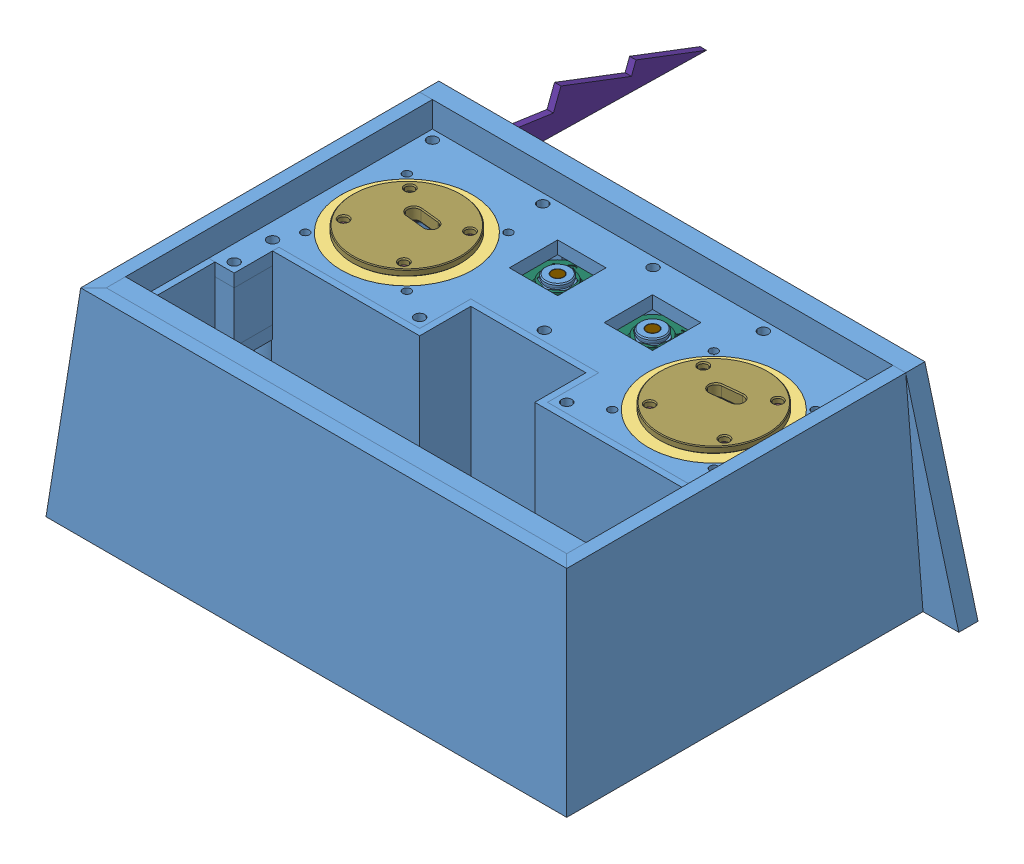
SolidWorks assembly 2WD Swerve Wedge Assembly, configuration Default. Lengths in mm.
Overall size (315.4 113.42 364.58).
92 component instances, 37 part files, 30 mates.
Components (placement in the parent):
- 2WD Swerve Wedge-1: 2WD Swerve Wedge [Default] at origin size (294.05 98.42 218.16)
- Manufacture Ready Swerve_Double Gearbox Wheel_Assem-1: Manufacture Ready Swerve_Double Gearbox Wheel_Assem [Default] at (-76.2 25.4 -25.4) x (0.105706 0 -0.994397) z (0.994397 0 0.105706) size (83.94 95.25 79.69)
  - PROPDRIVE 2836-1: PROPDRIVE 2836 [Default] at (-7.34 47.9628 0) x (0 0.80165 -0.597794) z (0 0.597794 0.80165) size (28 45.1 28)
  - Zoro Bearing 50mmID 65mm OD 7mmWidth-1: Zoro Bearing 50mmID 65mm OD 7mmWidth [Default] at (0 63.175 0) x (0.965482 0 -0.260469) z (0.260469 0 0.965482) size (65 7 65)
  - Zoro Bearing 50mmID 65mm OD 7mmWidth-2: Zoro Bearing 50mmID 65mm OD 7mmWidth [Default] at (0 32.075 0) x (0.000165 0 -1) z (1 0 0.000165) size (65 7 65)
  - Double Gearbox 36mm 19 to 1-2: Double Gearbox 36mm 19 to 1 [Default] at (-6.0895 0 0) x (0 0 1) z (0 1 0) size (36 76.01 36)
  - FL696ZZ-1: FL696ZZ [Default] at (30.7875 0 0) x (-1 0 0) z (0 -0.99717 0.07518) size (5 17 17)
  - Casted Swerve Wheel-1: Casted Swerve Wheel [Default] at (-0.4634 0 0) size (26.13 50.8 50.8)
  - Custom Input Shaft Pully-3: Custom Input Shaft Pully [Default] at (20.1995 0 0) x (0 0 1) z (0 1 0) size (19.98 11.18 19.98)
  - 5mm Pully Interface-1: 5mm Pully Interface [Default] at origin size (65.57 21.67 65.57)
  - Bottom Bearing Retainer-1: Bottom Bearing Retainer [Default] at origin size (56.35 4.76 56.35)
  - Drive Motor Face Mount-1: Drive Motor Face Mount [Default] at origin size (2.29 27.26 43.18)
  - Gearbox-Side Support-1: Gearbox-Side Support [Default] at origin size (6.35 34.92 28.57)
  - Inner Modual Lid-1: Inner Modual Lid [Default] at origin size (53.98 6.35 53.98)
  - Innermost Structure-1: Innermost Structure [Default] at origin size (50.34 38.64 53.98)
  - Left Motor Mount Retainer-1: Left Motor Mount Retainer [Default] at origin size (10.68 17.78 8.44)
  - Pully-Side Support-1: Pully-Side Support [Default] at origin size (6.35 34.92 28.57)
  - Wheel Support Mount Plate-1: Wheel Support Mount Plate [Default] at origin size (69.4 4.76 56.35)
  - Left Motor Mount Retainer-2: Left Motor Mount Retainer [Right] at origin size (10.68 17.78 8.44)
  - Custom Motor Output Shaft Pinion-3: Custom Motor Output Shaft Pinion [Default] at (19.431 47.9628 0) x (0 -0.974186 0.225748) z (0 0.225748 0.974186) size (16.43 12.7 16.28)
- 2845 3.17mm 2600kv Surpass-5: 2845 3.17mm 2600kv Surpass [Default] at (-30.46 28.575 41.275) x (0 -0.462995 0.886361) z (0 -0.886361 -0.462995) size (28 84.78 28)
- OVONIC - 1300mAh - 6S1P-1: OVONIC - 1300mAh - 6S1P [Default] at (72.39 34.29 33.655) x (0 1 0) z (1 0 0) size (36.86 42.55 90.17)
- 36mm 47.1(263_1) gear box-1: 36mm 47.1(263_1) gear box [Default] at (-57.897 28.575 41.275) x (0 0.707107 -0.707107) z (0 0.707107 0.707107) size (52.63 77.16 52.63)
  - 251916mount_36mm gearbox.step-1: 251916mount_36mm gearbox.step [Default] at (0 2.413 0) size (52.63 6.35 52.63)
  - 36mm 47.1(263_1) gear box.step-1: 36mm 47.1(263_1) gear box.step [Default] at origin size (36 45.1 36)
  - 36mm 47.1(263_1) gear box-0.step-1: 36mm 47.1(263_1) gear box-0.step [Default] at origin size (36 10.13 36)
  - 36mm 47.1(263_1) gear box-1.step-1: 36mm 47.1(263_1) gear box-1.step [Default] at origin size (8 20 8)
- DartBox V2 6mm Shaft-1: DartBox V2 6mm Shaft [Default] at (-8.1552 -10.937 -48.4676) x (-0.054657 0 -0.998505) z (0 1 0) size (21.95 21.95 72.3)
  - DartBox V2 6mm Shaft.stp-1: DartBox V2 6mm Shaft.stp [Default] at origin size (21.95 21.95 72.3)
    - DartBox V2 Drive 6mm Output.stp-1: DartBox V2 Drive 6mm Output.stp [Default] at (0 15.4164 54.362) x (0 1 0) z (0 0 1) size (21.95 21.95 42.9)
      - Ring Gear.stp-1: Ring Gear.stp [Default] at (-10.101 0.0152 -54.1116) x (0 -1 0) z (0 0 1) size (21.95 21.95 40.4)
        - Front Plate.stp-1: Front Plate.stp [Default] at (0.0152 10.101 56.6116) x (0 1 0) z (1 0 0) size (21.95 30.5 21.95)
          - Shaft.stp-1: Shaft.stp [Default] x (-0.819152 0 -0.573576) z (0.573576 0 -0.819152) size (7.4 30.3 6.7)
            - Retaining Ring.stp-1: Retaining Ring.stp [Default] at (0 16.65 0) x (-1 0 0) z (0 -1 0) size (7.4 6.16 0.5)
            - Shaft-0.stp-1: Shaft-0.stp [Default] at origin size (6 30.3 6)
          - Front Plate-1.stp-1: Front Plate-1.stp [Default] at origin size (21.95 6.5 21.95)
          - Front Plate-2.stp-1: Front Plate-2.stp [Default] at origin size (9.5 6 9.5)
        - Ring Gear Body.stp-1: Ring Gear Body.stp [Default] at (0.0152 10.101 56.6116) x (0 1 0) z (1 0 0) size (16.5 10.4 16.5)
      - Motor Mount Plate.stp-1: Motor Mount Plate.stp [Default] at (0 0 2.5) x (1 0 0) z (0 -1 0) size (21.95 3.5 21.95)
      - Screws M2 x 14mm.stp-1: Screws M2 x 14mm.stp [Default] at (6.364 6.364 0.9) size (3.4 3.4 15.61)
      - Screws M2 x 14mm.stp-2: Screws M2 x 14mm.stp [Default] at (-6.364 6.364 0.9) x (0 1 0) z (0 0 1) size (3.4 3.4 15.61)
      - Screws M2 x 14mm.stp-3: Screws M2 x 14mm.stp [Default] at (-6.364 -6.364 0.9) x (-1 0 0) z (0 0 1) size (3.4 3.4 15.61)
      - Screws M2 x 14mm.stp-4: Screws M2 x 14mm.stp [Default] at (6.364 -6.364 0.9) x (0 -1 0) z (0 0 1) size (3.4 3.4 15.61)
    - DartBox 130 motor.stp-1: DartBox 130 motor.stp [Default] at (0 15.4164 54.362) x (1 0 0) z (0 0 -1) size (15.5 20.4 34.9)
- Manufacture Ready Swerve_Double Gearbox Wheel_Assem-8: Manufacture Ready Swerve_Double Gearbox Wheel_Assem [Default] at (76.2 25.4 -25.4) x (-0.105706 0 -0.994397) z (0.994397 0 -0.105706) size (83.94 95.25 79.69)
  - PROPDRIVE 2836-1: PROPDRIVE 2836 [Default] at (-7.34 47.9628 0) x (0 0.80165 -0.597794) z (0 0.597794 0.80165) size (28 45.1 28)
  - Zoro Bearing 50mmID 65mm OD 7mmWidth-1: Zoro Bearing 50mmID 65mm OD 7mmWidth [Default] at (0 63.175 0) x (0.965482 0 -0.260469) z (0.260469 0 0.965482) size (65 7 65)
  - Zoro Bearing 50mmID 65mm OD 7mmWidth-2: Zoro Bearing 50mmID 65mm OD 7mmWidth [Default] at (0 32.075 0) x (0.000165 0 -1) z (1 0 0.000165) size (65 7 65)
  - Double Gearbox 36mm 19 to 1-2: Double Gearbox 36mm 19 to 1 [Default] at (-6.0895 0 0) x (0 0 1) z (0 1 0) size (36 76.01 36)
  - FL696ZZ-1: FL696ZZ [Default] at (30.7875 0 0) x (-1 0 0) z (0 -0.99717 0.07518) size (5 17 17)
  - Casted Swerve Wheel-1: Casted Swerve Wheel [Default] at (-0.4634 0 0) size (26.13 50.8 50.8)
  - Custom Input Shaft Pully-3: Custom Input Shaft Pully [Default] at (20.1995 0 0) x (0 0 1) z (0 1 0) size (19.98 11.18 19.98)
  - 5mm Pully Interface-1: 5mm Pully Interface [Default] at origin size (65.57 21.67 65.57)
  - Bottom Bearing Retainer-1: Bottom Bearing Retainer [Default] at origin size (56.35 4.76 56.35)
  - Drive Motor Face Mount-1: Drive Motor Face Mount [Default] at origin size (2.29 27.26 43.18)
  - Gearbox-Side Support-1: Gearbox-Side Support [Default] at origin size (6.35 34.92 28.57)
  - Inner Modual Lid-1: Inner Modual Lid [Default] at origin size (53.98 6.35 53.98)
  - Innermost Structure-1: Innermost Structure [Default] at origin size (50.34 38.64 53.98)
  - Left Motor Mount Retainer-1: Left Motor Mount Retainer [Default] at origin size (10.68 17.78 8.44)
  - Pully-Side Support-1: Pully-Side Support [Default] at origin size (6.35 34.92 28.57)
  - Wheel Support Mount Plate-1: Wheel Support Mount Plate [Default] at origin size (69.4 4.76 56.35)
  - Left Motor Mount Retainer-2: Left Motor Mount Retainer [Right] at origin size (10.68 17.78 8.44)
  - Custom Motor Output Shaft Pinion-3: Custom Motor Output Shaft Pinion [Default] at (19.431 47.9628 0) x (0 -0.974186 0.225748) z (0 0.225748 0.974186) size (16.43 12.7 16.28)
- DartBox V2 6mm Shaft-2: DartBox V2 6mm Shaft [Default] at (38.9419 -10.937 -46.7824) x (0.054657 0 -0.998505) z (0 1 0) size (21.95 21.95 72.3)
  - DartBox V2 6mm Shaft.stp-1: DartBox V2 6mm Shaft.stp [Default] at origin size (21.95 21.95 72.3)
    - DartBox V2 Drive 6mm Output.stp-1: DartBox V2 Drive 6mm Output.stp [Default] at (0 15.4164 54.362) x (0 1 0) z (0 0 1) size (21.95 21.95 42.9)
      - Ring Gear.stp-1: Ring Gear.stp [Default] at (-10.101 0.0152 -54.1116) x (0 -1 0) z (0 0 1) size (21.95 21.95 40.4)
        - Front Plate.stp-1: Front Plate.stp [Default] at (0.0152 10.101 56.6116) x (0 1 0) z (1 0 0) size (21.95 30.5 21.95)
          - Shaft.stp-1: Shaft.stp [Default] x (-0.819152 0 -0.573576) z (0.573576 0 -0.819152) size (7.4 30.3 6.7)
            - Retaining Ring.stp-1: Retaining Ring.stp [Default] at (0 16.65 0) x (-1 0 0) z (0 -1 0) size (7.4 6.16 0.5)
            - Shaft-0.stp-1: Shaft-0.stp [Default] at origin size (6 30.3 6)
          - Front Plate-1.stp-1: Front Plate-1.stp [Default] at origin size (21.95 6.5 21.95)
          - Front Plate-2.stp-1: Front Plate-2.stp [Default] at origin size (9.5 6 9.5)
        - Ring Gear Body.stp-1: Ring Gear Body.stp [Default] at (0.0152 10.101 56.6116) x (0 1 0) z (1 0 0) size (16.5 10.4 16.5)
      - Motor Mount Plate.stp-1: Motor Mount Plate.stp [Default] at (0 0 2.5) x (1 0 0) z (0 -1 0) size (21.95 3.5 21.95)
      - Screws M2 x 14mm.stp-1: Screws M2 x 14mm.stp [Default] at (6.364 6.364 0.9) size (3.4 3.4 15.61)
      - Screws M2 x 14mm.stp-2: Screws M2 x 14mm.stp [Default] at (-6.364 6.364 0.9) x (0 1 0) z (0 0 1) size (3.4 3.4 15.61)
      - Screws M2 x 14mm.stp-3: Screws M2 x 14mm.stp [Default] at (-6.364 -6.364 0.9) x (-1 0 0) z (0 0 1) size (3.4 3.4 15.61)
      - Screws M2 x 14mm.stp-4: Screws M2 x 14mm.stp [Default] at (6.364 -6.364 0.9) x (0 -1 0) z (0 0 1) size (3.4 3.4 15.61)
    - DartBox 130 motor.stp-1: DartBox 130 motor.stp [Default] at (0 15.4164 54.362) x (1 0 0) z (0 0 -1) size (15.5 20.4 34.9)
- RB Standoff_-2: RB Standoff_ [1000L] at (-87.3125 73.025 -30.1625) size (9.53 25.4 9.53)
- RB Standoff_-3: RB Standoff_ [1000L] at (87.3125 73.025 -30.1625) x (-1 0 0) z (0 0 -1) size (9.53 25.4 9.53)
- Proto Swerve Turn Pinion 5mm HTD Pulley-1: Proto Swerve Turn Pinion 5mm HTD Pulley [Default] at (-23.5486 73.9232 -47.625) x (0.789666 0 -0.613537) z (0.613537 0 0.789666) size (31.44 23.6 31.44)
- Proto Swerve Turn Pinion 5mm HTD Pulley-2: Proto Swerve Turn Pinion 5mm HTD Pulley [Default] at (23.5486 73.9232 -47.625) x (0.789666 0 0.613537) z (-0.613537 0 0.789666) size (31.44 23.6 31.44)
- RB Standoff_-11: RB Standoff_ [1000L] at (-36.5125 73.025 7.9375) x (0.918365 0 -0.395734) z (0.395734 0 0.918365) size (9.53 25.4 9.53)
- RB Standoff_-14: RB Standoff_ [1000L] at (36.5125 73.025 7.9375) x (-0.918365 0 -0.395734) z (0.395734 0 -0.918365) size (9.53 25.4 9.53)
- T81H-RM41.stp-1: T81H-RM41.stp [Default] at (-119.475 28.575 41.275) x (0 0.018679 0.999826) z (-1 0 0) size (20.32 20.32 20.32)
- 4wd Swerve Finger-1: 4wd Swerve Finger [Default] at (-122.015 28.575 41.275) x (0 0.018679 0.999826) z (0 -0.999826 0.018679) size (327.25 46.36 44.9)
- AS5600 Encoder Magnet-1: AS5600 Encoder Magnet [Default] at (-23.5486 88.2942 -47.625) size (6 2.5 6)
- Custom Motor Output Shaft-1: Custom Motor Output Shaft [Default] at (-23.5486 76.2346 -47.625) x (0.377103 0 -0.926171) z (0 -1 0) size (12.7 13.75 26.62)
- Custom Motor Output Shaft-2: Custom Motor Output Shaft [Default] at (23.5486 76.2346 -47.625) x (-0.377103 0 -0.926171) z (0 1 0) size (12.7 13.75 26.62)
- AS5600 Encoder Magnet-2: AS5600 Encoder Magnet [Default] at (23.5486 88.2942 -47.625) x (-1 0 0) z (0 0 -1) size (6 2.5 6)
Mates (geometry in assembly coordinates):
- Coincident1: coincident aligned: plane of 2WD Swerve Wedge-1 through (0 0 0) normal (0 0 1)
- Coincident2: coincident aligned: plane of 2WD Swerve Wedge-1 through (0 0 0) normal (0 1 0)
- Coincident3: coincident aligned: plane of 2WD Swerve Wedge-1 through (0 0 0) normal (1 0 0)
- Coincident4: coincident aligned: plane of 2WD Swerve Wedge-1 through (0 92.075 0) normal (0 1 0); plane of Manufacture Ready Swerve_Double Gearbox Wheel_Assem-1/Zoro Bearing 50mmID 65mm OD 7mmWidth-1 through (-76.2 92.075 -25.4) normal (0 1 0)
- Concentric1: concentric anti-aligned: cylinder of 2WD Swerve Wedge-1 through (-76.2 85.725 -25.4) axis (0 1 0) radius 32.5; cylinder of Manufacture Ready Swerve_Double Gearbox Wheel_Assem-1/Zoro Bearing 50mmID 65mm OD 7mmWidth-1 through (-76.2 92.075 -25.4) axis (0 -1 0) radius 32.5
- Coincident10: coincident anti-aligned: plane of 2845 3.17mm 2600kv Surpass-5 through (-53.96 28.575 41.275) normal (-1 0 0); plane of 36mm 47.1(263_1) gear box-1/251916mount_36mm gearbox.step-1 through (-53.96 28.575 41.275) normal (1 0 0)
- Concentric3: concentric aligned: cylinder of 2845 3.17mm 2600kv Surpass-5 through (-30.46 28.575 41.275) axis (-1 0 0) radius 14; cylinder of 36mm 47.1(263_1) gear box-1/36mm 47.1(263_1) gear box.step-1 through (-57.897 28.575 41.275) axis (-1 0 0) radius 18
- Coincident12: coincident: line of 2WD Swerve Wedge-1 through (-111.125 0 59.275) axis (0 0 -1); plane of 36mm 47.1(263_1) gear box-1/36mm 47.1(263_1) gear box-0.step-1 through (-111.125 28.575 41.275) normal (-1 0 0)
- Coincident18: coincident aligned: plane of 2WD Swerve Wedge-1 through (0 60.325 0) normal (0 1 0); plane of DartBox V2 6mm Shaft-1/DartBox V2 6mm Shaft.stp-1/DartBox V2 Drive 6mm Output.stp-1/Ring Gear.stp-1/Front Plate.stp-1/Front Plate-1.stp-1 through (-23.5486 60.325 -47.625) normal (0 1 0)
- Concentric6: concentric aligned: cylinder of DartBox V2 6mm Shaft-1/DartBox V2 6mm Shaft.stp-1/DartBox V2 Drive 6mm Output.stp-1/Ring Gear.stp-1/Front Plate.stp-1/Front Plate-1.stp-1 through (-23.5486 56.325 -47.625) axis (0 1 0) radius 10.975; cylinder of 2WD Swerve Wedge-1 through (-23.5486 53.975 -47.625) axis (0 1 0) radius 10.9728
- Coincident23: coincident anti-aligned: plane of 2WD Swerve Wedge-1 through (0 60.325 0) normal (0 1 0); plane of RB Standoff_-2 through (-87.3125 60.325 -30.1625) normal (0 -1 0)
- Coincident26: coincident anti-aligned: plane of 2WD Swerve Wedge-1 through (0 60.325 0) normal (0 1 0); plane of RB Standoff_-11 through (-36.5125 60.325 7.9375) normal (0 -1 0)
- Concentric14: concentric anti-aligned: cylinder of 2WD Swerve Wedge-1 through (-36.5125 53.975 7.9375) axis (0 1 0) radius 2.5527; cylinder of RB Standoff_-11 through (-36.5125 85.725 7.9375) axis (0 -1 0) radius 4.7625
- Concentric16: concentric anti-aligned: cylinder of 36mm 47.1(263_1) gear box-1/36mm 47.1(263_1) gear box-1.step-1 through (-111.125 28.575 41.275) axis (-1 0 0) radius 4; line of T81H-RM41.stp-1 through (-140.811 28.575 41.275) axis (1 0 0)
- Distance3: distance = 6.35 mm aligned: plane of T81H-RM41.stp-1 through (-119.475 28.575 41.275) normal (-1 0 0); plane of 36mm 47.1(263_1) gear box-1/36mm 47.1(263_1) gear box-0.step-1 through (-113.125 28.575 41.275) normal (-1 0 0)
- Concentric21: concentric aligned: line of T81H-RM41.stp-1 through (-140.811 28.575 41.275) axis (1 0 0); cylinder of 4wd Swerve Finger-1 through (-139.795 28.575 41.275) axis (1 0 0) radius 9.525
- Tangent2: tangent: plane of assembly; face of T81H-RM41.stp-1; plane of 4wd Swerve Finger-1 through (-139.795 28.575 41.275) normal (-1 0 0)
- Concentric22: concentric anti-aligned: cylinder of DartBox V2 6mm Shaft-1/DartBox V2 6mm Shaft.stp-1/DartBox V2 Drive 6mm Output.stp-1/Ring Gear.stp-1/Front Plate.stp-1/Shaft.stp-1/Shaft-0.stp-1 through (-23.5486 62.325 -47.625) axis (0 1 0) radius 3; cylinder of Custom Motor Output Shaft-1 through (-23.5486 89.5442 -47.625) axis (0 -1 0) radius 2.9972
- Coincident32: coincident anti-aligned: plane of DartBox V2 6mm Shaft-1/DartBox V2 6mm Shaft.stp-1/DartBox V2 Drive 6mm Output.stp-1/Ring Gear.stp-1/Front Plate.stp-1/Shaft.stp-1/Retaining Ring.stp-1 through (-23.5486 62.925 -47.625) normal (0 1 0); plane of Custom Motor Output Shaft-1 through (-18.1379 62.925 -45.422) normal (0 -1 0)
- Concentric23: concentric anti-aligned: cylinder of Proto Swerve Turn Pinion 5mm HTD Pulley-1 through (-23.5486 86.0212 -47.625) axis (0 1 0) radius 15.7209; cylinder of Custom Motor Output Shaft-1 through (-23.5486 89.5442 -47.625) axis (0 -1 0) radius 2.9972
- Coincident36: coincident anti-aligned: plane of Proto Swerve Turn Pinion 5mm HTD Pulley-1 through (-17.7585 84.4388 -52.1237) normal (-0.990639 0 0.136505); plane of Custom Motor Output Shaft-1 through (-17.6184 65.465 -51.1074) normal (0.990639 0 -0.136505)
- Coincident37: coincident aligned: plane of Proto Swerve Turn Pinion 5mm HTD Pulley-1 through (-23.5486 87.0042 -47.625) normal (0 1 0); plane of Custom Motor Output Shaft-1 through (-23.5486 87.0042 -47.625) normal (0 1 0)
- Coincident38: coincident aligned: plane of AS5600 Encoder Magnet-1 through (-23.5486 89.5442 -47.625) normal (0 1 0); plane of Custom Motor Output Shaft-1 through (-18.1379 89.5442 -45.422) normal (0 1 0)
- Concentric24: concentric aligned: cylinder of AS5600 Encoder Magnet-1 through (-23.5486 89.5442 -47.625) axis (0 -1 0) radius 3; cylinder of Custom Motor Output Shaft-1 through (-23.5486 89.5442 -47.625) axis (0 -1 0) radius 2.9972
- Coincident40: coincident anti-aligned: plane of 2WD Swerve Wedge-1 through (0 0 76.2) normal (0 0 -1); plane of OVONIC - 1300mAh - 6S1P-1 through (72.39 34.29 76.2) normal (0 0 1)
- Distance4: distance = 15.875 mm: plane of assembly through (0 0 0) normal (0 1 0); plane of assembly; plane of OVONIC - 1300mAh - 6S1P-1 through (33.655 15.875 76.2) normal (0 -1 0)
- Coincident43: coincident anti-aligned: plane of 2WD Swerve Wedge-1 through (111.125 0 0) normal (-1 0 0); plane of OVONIC - 1300mAh - 6S1P-1 through (111.125 15.875 76.2) normal (1 0 0)
- Concentric25: concentric aligned: cylinder of 2WD Swerve Wedge-1 through (-39.7757 13.335 56.515) axis (-1 0 0) radius 1.5875; cylinder of 36mm 47.1(263_1) gear box-1/251916mount_36mm gearbox.step-1 through (-53.325 13.335 56.515) axis (-1 0 0) radius 1.3843
- Concentric26: concentric aligned: cylinder of 2WD Swerve Wedge-1 through (-39.7757 13.335 26.035) axis (-1 0 0) radius 1.5875; cylinder of 36mm 47.1(263_1) gear box-1/251916mount_36mm gearbox.step-1 through (-53.325 13.335 26.035) axis (-1 0 0) radius 1.3843
- Coincident44: coincident anti-aligned: plane of T81H-RM41.stp-1 through (-127.095 38.8548 47.5909) normal (0 0.999826 -0.018679); plane of 4wd Swerve Finger-1 through (-129.635 38.5435 30.927) normal (0 -0.999826 0.018679)
